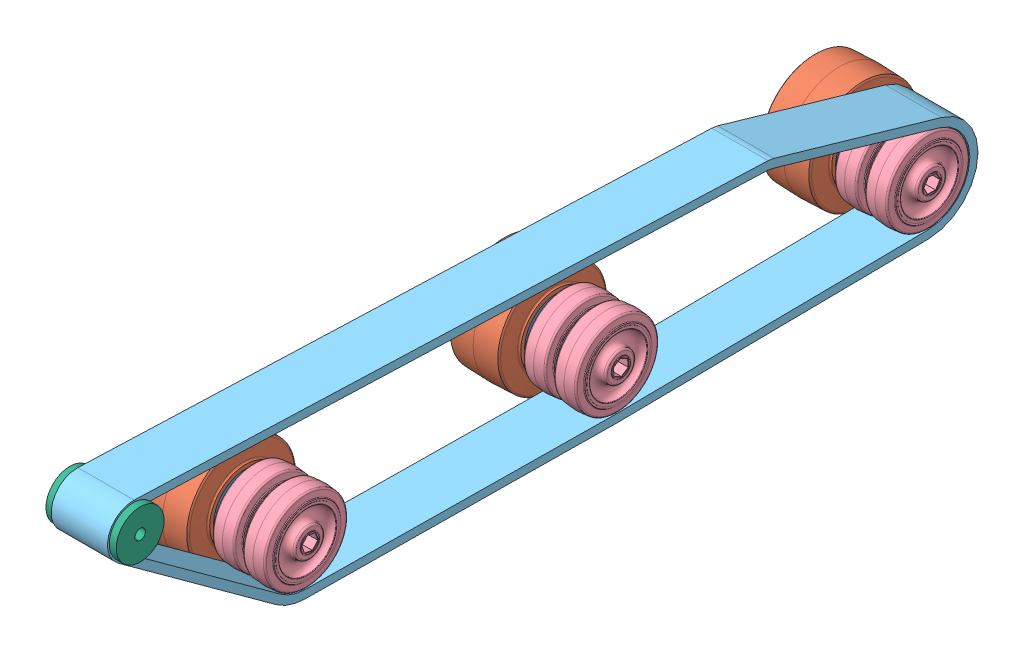
SolidWorks assembly 0001- 01 - 1040 WHEEL ASSEMBLY, configuration Default. Lengths in mm.
Overall size (115.1 373.88 795.79).
21 component instances, 7 part files, 32 mates.
Components (placement in the parent):
- 0001- 01 - 0001 Reference Geometry-1: 0001- 01 - 0001 Reference Geometry [Default] at origin size (111.12 355.6 787.4) (hidden)
- Colson - 4 x 2 Hex-1: Colson - 4 x 2 Hex [Default] at (28.9766 50.8 -455.7037) x (1 0 0) z (0 -0.557084 0.830456) size (57.95 99.57 99.57)
  - Colson - 4 x 2 Hex 03-1: Colson - 4 x 2 Hex 03 [Default] at origin size (55.55 82.55 82.55)
  - Colson - 4 x 2 Hex 01-1: Colson - 4 x 2 Hex 01 [Default] at origin size (50.8 99.57 99.57)
  - Colson - 4 x 2 Hex 02-1: Colson - 4 x 2 Hex 02 [Default] x (0 0 1) z (-1 0 0) size (50.79 50.79 57.95)
- Colson - 4 x 2 Hex-2: Colson - 4 x 2 Hex [Default] at (28.9766 53.975 -736.6) x (1 0 0) z (0 -0.049345 -0.998782) size (57.95 99.57 99.57)
  - Colson - 4 x 2 Hex 03-1: Colson - 4 x 2 Hex 03 [Default] at origin size (55.55 82.55 82.55)
  - Colson - 4 x 2 Hex 01-1: Colson - 4 x 2 Hex 01 [Default] at origin size (50.8 99.57 99.57)
  - Colson - 4 x 2 Hex 02-1: Colson - 4 x 2 Hex 02 [Default] x (0 0 1) z (-1 0 0) size (50.79 50.79 57.95)
- Colson - 4 x 2 Hex-3: Colson - 4 x 2 Hex [Default] at (28.9766 53.975 -174.8073) x (1 0 0) z (0 0.745926 -0.666029) size (57.95 99.57 99.57)
  - Colson - 4 x 2 Hex 03-1: Colson - 4 x 2 Hex 03 [Default] at origin size (55.55 82.55 82.55)
  - Colson - 4 x 2 Hex 01-1: Colson - 4 x 2 Hex 01 [Default] at origin size (50.8 99.57 99.57)
  - Colson - 4 x 2 Hex 02-1: Colson - 4 x 2 Hex 02 [Default] x (0 0 1) z (-1 0 0) size (50.79 50.79 57.95)
- Colson - 3 x 0.875 Hex-1: Colson - 3 x 0.875 Hex [Default] at (71.7469 53.975 -174.8073) x (0 0.203834 0.979005) z (-1 0 0) size (76.2 76.2 27.59)
- Colson - 3 x 0.875 Hex-2: Colson - 3 x 0.875 Hex [Default] at (99.3345 53.975 -174.8073) x (0 0.203834 0.979005) z (-1 0 0) size (76.2 76.2 27.59)
- Colson - 3 x 0.875 Hex-3: Colson - 3 x 0.875 Hex [Default] at (71.7469 50.8 -455.7037) x (0 -0.557084 0.830456) z (-1 0 0) size (76.2 76.2 27.59)
- Colson - 3 x 0.875 Hex-4: Colson - 3 x 0.875 Hex [Default] at (99.3345 50.8 -455.7037) x (0 -0.557084 0.830456) z (-1 0 0) size (76.2 76.2 27.59)
- Colson - 3 x 0.875 Hex-5: Colson - 3 x 0.875 Hex [Default] at (99.3345 53.975 -736.6) x (0 -0.049345 -0.998782) z (-1 0 0) size (76.2 76.2 27.59)
- Colson - 3 x 0.875 Hex-6: Colson - 3 x 0.875 Hex [Default] at (71.7469 53.975 -736.6) x (0 -0.049345 -0.998782) z (-1 0 0) size (76.2 76.2 27.59)
- 0001- 01 - 1041 Tread-1: 0001- 01 - 1041 Tread [Default] at (57.9532 0 0) size (50.8 157.69 786.26)
- 0001- 01 - 1042 Top Pulley-1: 0001- 01 - 1042 Top Pulley [Default] at (51.6032 139.7817 -19.05) x (1 0 0) z (0 0.971922 -0.235302) size (63.5 43.18 43.18)
Mates (geometry in assembly coordinates):
- Coincident1: coincident aligned: plane of 0001- 01 - 0001 Reference Geometry-1 through (0 0 0) normal (0 0 1); plane of assembly through (0 0 0) normal (0 0 1)
- Coincident2: coincident aligned: plane of 0001- 01 - 0001 Reference Geometry-1 through (0 0 0) normal (0 1 0); plane of assembly through (0 0 0) normal (0 1 0)
- Coincident3: coincident aligned: plane of 0001- 01 - 0001 Reference Geometry-1 through (0 0 0) normal (1 0 0); plane of assembly through (0 0 0) normal (1 0 0)
- Coincident4: coincident anti-aligned: plane of Colson - 4 x 2 Hex-3/Colson - 4 x 2 Hex 02-1 through (0 53.975 -174.8073) normal (-1 0 0); plane of assembly through (0 0 0) normal (1 0 0)
- Concentric1: concentric anti-aligned: circle of 0001- 01 - 0001 Reference Geometry-1; circle of Colson - 4 x 2 Hex-3/Colson - 4 x 2 Hex 01-1
- Coincident5: coincident anti-aligned: plane of Colson - 4 x 2 Hex-1/Colson - 4 x 2 Hex 02-1 through (0 50.8 -455.7037) normal (-1 0 0); plane of assembly through (0 0 0) normal (1 0 0)
- Concentric2: concentric anti-aligned: circle of 0001- 01 - 0001 Reference Geometry-1; circle of Colson - 4 x 2 Hex-1/Colson - 4 x 2 Hex 01-1
- Concentric3: concentric anti-aligned: circle of 0001- 01 - 0001 Reference Geometry-1; circle of Colson - 4 x 2 Hex-2/Colson - 4 x 2 Hex 01-1
- Coincident6: coincident anti-aligned: plane of Colson - 4 x 2 Hex-2/Colson - 4 x 2 Hex 02-1 through (0 53.975 -736.6) normal (-1 0 0); plane of assembly through (0 0 0) normal (1 0 0)
- Coincident7: coincident anti-aligned: plane of Colson - 4 x 2 Hex-3/Colson - 4 x 2 Hex 02-1 through (57.9532 53.975 -174.8073) normal (1 0 0); plane of Colson - 3 x 0.875 Hex-1 through (57.9532 53.975 -174.8073) normal (-1 0 0)
- Concentric4: concentric anti-aligned: cone of Colson - 4 x 2 Hex-3/Colson - 4 x 2 Hex 02-1 through (30.774 53.975 -174.8073) axis (1 0 0); cone of Colson - 3 x 0.875 Hex-1 through (58.6532 53.975 -174.8073) axis (-1 0 0)
- Coincident9: coincident aligned: plane of Colson - 4 x 2 Hex-3/Colson - 4 x 2 Hex 02-1 through (0.3 52.4774 -182.0001) normal (0 0.666029 0.745926); plane of Colson - 3 x 0.875 Hex-1 through (58.2532 52.4774 -182.0001) normal (0 0.666029 0.745926)
- Coincident10: coincident anti-aligned: plane of Colson - 3 x 0.875 Hex-1 through (85.5407 53.975 -174.8073) normal (1 0 0); plane of Colson - 3 x 0.875 Hex-2 through (85.5407 53.975 -174.8073) normal (-1 0 0)
- Concentric5: concentric anti-aligned: cone of Colson - 3 x 0.875 Hex-1 through (84.8406 53.975 -174.8073) axis (1 0 0); cone of Colson - 3 x 0.875 Hex-2 through (86.2408 53.975 -174.8073) axis (-1 0 0)
- Coincident12: coincident anti-aligned: plane of Colson - 4 x 2 Hex-1/Colson - 4 x 2 Hex 02-1 through (57.9532 50.8 -455.7037) normal (1 0 0); plane of Colson - 3 x 0.875 Hex-3 through (57.9532 50.8 -455.7037) normal (-1 0 0)
- Concentric6: concentric anti-aligned: cone of Colson - 4 x 2 Hex-1/Colson - 4 x 2 Hex 02-1 through (30.774 50.8 -455.7037) axis (1 0 0); cone of Colson - 3 x 0.875 Hex-3 through (58.6532 50.8 -455.7037) axis (-1 0 0)
- Coincident14: coincident aligned: plane of Colson - 3 x 0.875 Hex-1 through (58.2532 52.4774 -182.0001) normal (0 0.666029 0.745926); plane of Colson - 3 x 0.875 Hex-2 through (85.8407 52.4774 -182.0001) normal (0 0.666029 0.745926)
- Coincident15: coincident anti-aligned: plane of Colson - 3 x 0.875 Hex-3 through (85.5407 50.8 -455.7037) normal (1 0 0); plane of Colson - 3 x 0.875 Hex-4 through (85.5407 50.8 -455.7037) normal (-1 0 0)
- Concentric7: concentric anti-aligned: cone of Colson - 3 x 0.875 Hex-3 through (84.8406 50.8 -455.7037) axis (1 0 0); cone of Colson - 3 x 0.875 Hex-4 through (86.2408 50.8 -455.7037) axis (-1 0 0)
- Coincident17: coincident aligned: plane of Colson - 3 x 0.875 Hex-3 through (58.2532 54.8929 -461.805) normal (0 -0.06722 0.997738); plane of Colson - 3 x 0.875 Hex-4 through (85.8407 54.8929 -461.805) normal (0 -0.06722 0.997738)
- Coincident18: coincident aligned: plane of Colson - 4 x 2 Hex-1/Colson - 4 x 2 Hex 02-1 through (0.3 54.8929 -461.805) normal (0 -0.06722 0.997738); plane of Colson - 3 x 0.875 Hex-3 through (58.2532 54.8929 -461.805) normal (0 -0.06722 0.997738)
- Coincident19: coincident anti-aligned: plane of Colson - 4 x 2 Hex-2/Colson - 4 x 2 Hex 02-1 through (57.9532 53.975 -736.6) normal (1 0 0); plane of Colson - 3 x 0.875 Hex-6 through (57.9532 53.975 -736.6) normal (-1 0 0)
- Concentric8: concentric anti-aligned: cone of Colson - 4 x 2 Hex-2/Colson - 4 x 2 Hex 02-1 through (30.774 53.975 -736.6) axis (1 0 0); cone of Colson - 3 x 0.875 Hex-6 through (58.6532 53.975 -736.6) axis (-1 0 0)
- Concentric9: concentric anti-aligned: cone of Colson - 3 x 0.875 Hex-5 through (86.2408 53.975 -736.6) axis (-1 0 0); cone of Colson - 3 x 0.875 Hex-6 through (84.8406 53.975 -736.6) axis (1 0 0)
- Coincident22: coincident anti-aligned: plane of Colson - 3 x 0.875 Hex-5 through (85.5407 53.975 -736.6) normal (-1 0 0); plane of Colson - 3 x 0.875 Hex-6 through (85.5407 53.975 -736.6) normal (1 0 0)
- Coincident23: coincident aligned: plane of Colson - 4 x 2 Hex-2/Colson - 4 x 2 Hex 02-1 through (0.3 60.1487 -740.583) normal (0 -0.456657 0.889643); plane of Colson - 3 x 0.875 Hex-6 through (58.2532 60.1487 -740.583) normal (0 -0.456657 0.889643)
- Coincident24: coincident aligned: plane of Colson - 3 x 0.875 Hex-5 through (85.8407 60.1487 -740.583) normal (0 -0.456657 0.889643); plane of Colson - 3 x 0.875 Hex-6 through (58.2532 60.1487 -740.583) normal (0 -0.456657 0.889643)
- Coincident25: coincident aligned: plane of 0001- 01 - 1041 Tread-1 through (57.9532 0 0) normal (0 0 1); plane of assembly through (0 0 0) normal (0 0 1)
- Coincident26: coincident aligned: plane of 0001- 01 - 1041 Tread-1 through (57.9532 0 0) normal (0 1 0); plane of assembly through (0 0 0) normal (0 1 0)
- Coincident27: coincident aligned: plane of 0001- 01 - 1041 Tread-1 through (57.9532 0 0) normal (1 0 0); plane of assembly through (57.9532 0 0) normal (1 0 0)
- Coincident28: coincident anti-aligned: plane of 0001- 01 - 1041 Tread-1 through (57.9532 139.7817 -19.05) normal (-1 0 0); plane of 0001- 01 - 1042 Top Pulley-1 through (57.9532 139.7817 -19.05) normal (1 0 0)
- Concentric10: concentric aligned: cylinder of 0001- 01 - 1041 Tread-1 through (108.7532 139.7817 -19.05) axis (-1 0 0) radius 15.875; cylinder of 0001- 01 - 1042 Top Pulley-1 through (108.7532 139.7817 -19.05) axis (-1 0 0) radius 15.875
